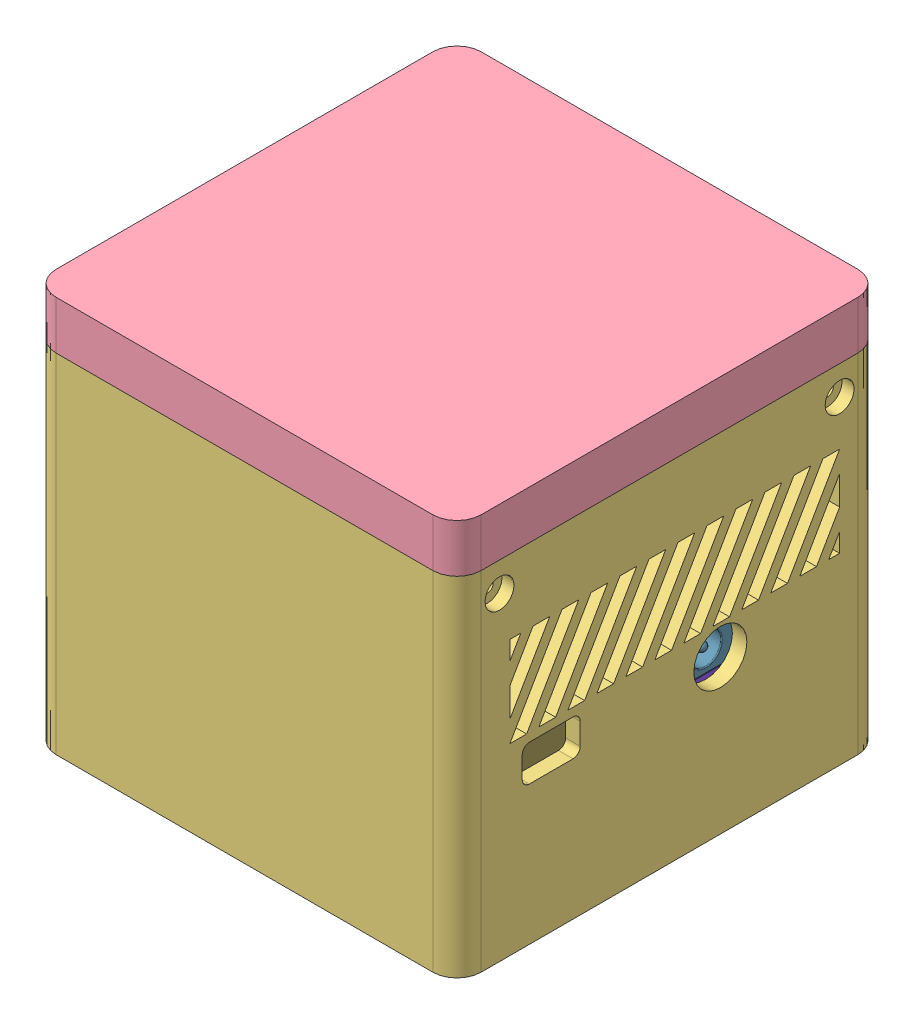
SolidWorks assembly 1219 ControlBox version, configuration 預設. Lengths in mm.
Overall size (88 82 106.01).
42 component instances, 34 part files, 73 mates.
Components (placement in the parent):
- 1219 third floor-1: 1219 third floor [預設] at (8.7787 40.759 112.8702) x (1 0 0) z (0 0 -1) size (81.6 37.75 81.6)
- 1219 second floor-1: 1219 second floor [預設] at (8.7787 -23.241 112.8702) x (1 0 0) z (0 0 -1) size (81.6 8 81.6)
- 1219 ground-1: 1219 ground [預設] at (0.3623 -33.241 92.6228) size (88 72 88)
- 1219 roof-1: 1219 roof [預設] at (-3.5854 48.759 93.9882) x (1 0 0) z (0 0 -1) size (88 10 88)
- STM32 fixed board-1: STM32 fixed board [預設] at (7.9161 -18.241 103.3439) x (-1 0 0) z (0 1 0) size (70.08 30 1.8)
- The small Fixed board on the converter-1: The small Fixed board on the converter [預設] at (21.8123 17.059 74.3493) x (0 0 -1) z (-1 0 0) size (46.7 1.6 58.25)
- M3_20mm_pillar-1: M3_20mm_pillar [預設] at (12.0438 39.859 57) x (-0.990685 0 -0.13617) z (-0.13617 0 0.990685) size (6 22.8 6)
- M3_20mm_pillar-2: M3_20mm_pillar [預設] at (28.2938 39.859 87.2) x (0.837169 0 0.546944) z (0.546944 0 -0.837169) size (6 22.8 6)
- 12VLEDconnector-1: 12VLEDconnector [預設] at (41.8438 -2.8554 76.5711) x (0 1 0) z (-1 0 0) size (12 37 6.2)
- O2-1: O2 [預設] at (-12.6825 28.759 117.8445) x (-1 0 0) z (0 1 0) size (37 27 19)
- JQC3F-1: JQC3F [預設] at (-14.4789 35.759 60.4222) x (1 0 0.000244) z (0 -1 0) size (33.51 25.73 16.5)
- LM2596 DC to DC Buck Converter 3 A-1: LM2596 DC to DC Buck Converter 3 A [預設] at (20.1688 38.759 72.1) x (0 0 -1) z (-1 0 0) size (43.2 15.15 21.25)
  - LM2596 DC to DC Buck Converter 3 A.STEP-1: LM2596 DC to DC Buck Converter 3 A.STEP [預設] at origin size (43.2 15.15 21.25)
    - lm2596board.STEP-1: lm2596board.STEP [預設] at origin size (43.2 1.71 21.25)
    - smd100uF.STEP-1: smd100uF.STEP [預設] at (-17.25 2.55 0) x (0 0 -1) z (1 0 0) size (11.2 9.76 8.2)
    - smd220uF.STEP-1: smd220uF.STEP [預設] at (17.25 2.55 0) x (0 0 -1) z (1 0 0) size (11.2 9.76 8.2)
    - TrimmerW203.STEP-1: TrimmerW203.STEP [預設] at (4.6271 6.95 -9.1276) size (9.5 15.15 4.81)
    - smdS537diode.STEP-1: smdS537diode.STEP [預設] at (-9.35 1.75 8.875) x (-1 0 0) z (0 0 -1) size (6.5 2.06 2.5)
    - smdceramiccapacitor.STEP-1: smdceramiccapacitor.STEP [預設] at (-15 1.7 5.7969) x (0 0 1) z (-1 0 0) size (2.52 0.61 1.3)
    - smdceramiccapacitor.STEP-2: smdceramiccapacitor.STEP [預設] at (-1.3196 1.7 -5.2916) x (0 0 1) z (-1 0 0) size (2.52 0.61 1.3)
    - smdResistor331.STEP-1: smdResistor331.STEP [預設] at (-1.2696 1.7 -8.4665) x (0 0 1) z (-1 0 0) size (2.53 0.63 1.31)
    - smdResistor102.STEP-1: smdResistor102.STEP [預設] at (10.7771 1.7 -8.4665) x (0 0 -1) z (1 0 0) size (2.53 0.63 1.31)
    - smdLED.STEP-1: smdLED.STEP [預設] at (13.0521 1.75 -8.4701) x (0 0 -1) z (1 0 0) size (3.23 0.86 1.26)
    - smbInductor470.STEP-1: smbInductor470.STEP [預設] at (3.1271 2.1 3.175) size (12.5 7.41 12.5)
    - LM2596S.STEP-1: LM2596S.STEP [預設] at (-8.0627 1.8 -4.5407) size (9.8 4.61 14.95)
- SCD30_CO2-1: SCD30_CO2 [預設] at (27.7597 38.759 111.9487) x (1 0 0) z (0 -1 0) size (35 23 13)
- Gravity Dissolved Oxygen Sensor v1.0.step-1: Gravity Dissolved Oxygen Sensor v1.0.step [預設] at (20.5726 -17.241 68.5206) x (-0.001647 0 0.999999) z (0 1 0) size (63.5 32 13.2)
- PH-4502C.STEP-1: PH-4502C.STEP [預設] at (-10.49 -8.3658 14.8331) x (0.023795 0 -0.999717) z (0.999717 0 0.023795) size (69.21 20.03 32.26)
  - Board_ph.STEP-1: Board_ph.STEP [預設] at (-41.1248 -11.8752 -79.7631) size (42 1.6 32)
  - BNC_90.STEP-1: BNC_90.STEP [預設] at (-42.729 11.0976 0.372) x (-0.000016 0 -1) z (0 -1 0) size (13 30 18)
  - Trimpot multivoltas_Valor predeterminado.STEP-1: Trimpot multivoltas_Valor predeterminado.STEP [預設] at (-58.9938 -5.1252 9.5069) x (-1 0 0) z (0 0 -1) size (9.8 15.4 5)
  - Trimpot multivoltas_Valor predeterminado.STEP-2: Trimpot multivoltas_Valor predeterminado.STEP [預設] at (-44.5735 -5.1252 13.9129) size (9.8 15.4 5)
  - pin_header_6.STEP-1: pin_header_6.STEP [預設] at (-71.799 -14.5822 4.6019) size (10.45 8.64 15.24)
  - S08.stp.STEP-1: S08.stp.STEP [預設] at (-63.5983 -10.4552 -1.493) x (1 0 0) z (0 1 0) size (4.9 6 1.55)
  - S08.stp.STEP-2: S08.stp.STEP [預設] at (-47.5601 -10.4552 -15.9552) x (-0.008727 0 0.999962) z (0 1 0) size (4.9 6 1.55)
  - S08.stp.STEP-3: S08.stp.STEP [預設] at (-45.4779 -10.4552 -0.8959) x (-0.999848 0 -0.017452) z (0 1 0) size (4.9 6 1.55)
  - ptc.STEP-1: ptc.STEP [預設] at (-58.5127 -8.5499 -13.3623) x (0 -1 0) z (0 0 -1) size (11.73 9.76 5.87)
- STM32 Nucleo-32-1: STM32 Nucleo-32 [預設] at (17.5119 -16.441 114.2714) x (1 0 0) z (0 1 0) size (50.29 18.54 16)
- JQC3F -2-1: JQC3F -2 [預設] at (-15.4815 35.759 86.544) x (1 0 0.000244) z (0 -1 0) size (34 26.5 16.5)
- DC socket-1: DC socket [Default] at (45.0438 -1.491 76.492) x (0 1 0) z (1 0 0) size (9.4 15 14.3)
- YELLOW JST XH 3 PIN CONNECTOR - P 2.54mm - ANGLED.stp-1: YELLOW JST XH 3 PIN CONNECTOR - P 2.54mm - ANGLED.stp [預設] at (19.2438 12.609 53.8153) x (0 -1 0) z (1 0 0) size (8.73 7.46 10.34)
- YELLOW JST XH 4 PIN CONNECTOR - P 2.54mm - ANGLED.stp-1: YELLOW JST XH 4 PIN CONNECTOR - P 2.54mm - ANGLED.stp [預設] at (-12.5062 12.609 53.8153) x (0 -1 0) z (1 0 0) size (8.73 7.46 12.88)
Mates (geometry in assembly coordinates):
- 重合/共線/共點6: coincident anti-aligned: plane of 1219 ground-1 through (0.3623 -25.241 92.6228) normal (0 1 0); plane of 1219 second floor-1 through (8.7787 -25.241 112.8702) normal (0 -1 0)
- 重合/共線/共點8: coincident anti-aligned: plane of 1219 second floor-1 through (8.7787 -23.241 112.8702) normal (0 1 0); plane of EC and PH support-1 through (-14.5186 -23.241 69.2115) normal (0 -1 0)
- 重合/共線/共點9: coincident anti-aligned: plane of EC and PH support-2 through (26.7761 -17.241 71.7105) normal (0 1 0); plane of Gravity Dissolved Oxygen Sensor v1.0.step-1 through (20.5726 -17.241 68.5206) normal (0 -1 0)
- 同軸心1: concentric aligned: cylinder of 1219 second floor-1 through (8.0438 -23.24 86) axis (0 -1 0) radius 1.2; cylinder of Gravity Dissolved Oxygen Sensor v1.0.step-1 through (8.0438 -15.741 86) axis (0 -1 0) radius 1.5
- 重合/共線/共點10: coincident anti-aligned: plane of EC and PH support-1 through (-14.5186 -20.241 69.2115) normal (0 1 0); plane of PH-4502C.STEP-1/Board_ph.STEP-1 through (1.9974 -20.241 47.1083) normal (0 -1 0)
- 同軸心3: concentric aligned: cylinder of 1219 second floor-1 through (-0.9062 -23.24 85.05) axis (0 -1 0) radius 1.2; cylinder of PH-4502C.STEP-1/Board_ph.STEP-1 through (-0.9062 -18.641 85.05) axis (0 -1 0) radius 1.5
- 重合/共線/共點16: coincident anti-aligned: plane of STM32 fixed board-1 through (7.9161 -16.441 103.3439) normal (0 1 0); plane of STM32 Nucleo-32-1 through (17.5119 -16.441 114.2714) normal (0 -1 0)
- 同軸心13: concentric aligned: cylinder of 1219 third floor-1 through (-24.9562 40.759 124) axis (0 -1 0) radius 1.2; cylinder of O2-1 through (-24.9562 30.759 124) axis (0 -1 0) radius 1.6
- 同軸心17: concentric aligned: cylinder of 1219 third floor-1 through (2.0438 40.759 50) axis (0 -1 0) radius 1.2; circle of JQC3F-1
- 同軸心18: concentric anti-aligned: cylinder of 1219 third floor-1 through (2.0438 40.759 70.5) axis (0 -1 0) radius 1.2; cylinder of JQC3F-1 through (2.0438 34.259 70.5) axis (0 1 0) radius 1.5
- 重合/共線/共點20: coincident anti-aligned: plane of 1219 third floor-1 through (8.7787 38.759 112.8702) normal (0 -1 0); plane of SCD30_CO2-1 through (27.7597 38.759 111.9487) normal (0 1 0)
- 同軸心21: concentric aligned: cylinder of 1219 third floor-1 through (11.0938 40.759 115.5) axis (0 -1 0) radius 1; cylinder of SCD30_CO2-1 through (11.0938 38.76 115.5) axis (0 -1 0) radius 0.875
- 同軸心22: concentric aligned: cylinder of 1219 third floor-1 through (43.0438 40.759 99.31) axis (0 -1 0) radius 1; cylinder of SCD30_CO2-1 through (43.0438 38.76 99.31) axis (0 -1 0) radius 0.875
- 同軸心23: concentric anti-aligned: circle of 1219 third floor-1; cylinder of LM2596 DC to DC Buck Converter 3 A-1/LM2596 DC to DC Buck Converter 3 A.STEP-1/lm2596board.STEP-1 through (12.0438 37.059 57) axis (0 1 0) radius 1.475
- 同軸心24: concentric aligned: cylinder of 1219 third floor-1 through (28.2938 40.759 87.2) axis (0 -1 0) radius 1.2; circle of LM2596 DC to DC Buck Converter 3 A-1/LM2596 DC to DC Buck Converter 3 A.STEP-1/lm2596board.STEP-1
- 重合/共線/共點27: coincident anti-aligned: plane of 1219 second floor-1 through (8.7787 -23.241 112.8702) normal (0 1 0); plane of EC and PH support-3 through (25.441 -23.241 60.8804) normal (0 -1 0)
- 重合/共線/共點28: coincident anti-aligned: plane of EC and PH support-2 through (26.7761 -20.241 71.7105) normal (0 -1 0); plane of EC and PH support-3 through (25.441 -20.241 60.8804) normal (0 1 0)
- 同軸心27: concentric aligned: cylinder of LM2596 DC to DC Buck Converter 3 A-1/LM2596 DC to DC Buck Converter 3 A.STEP-1/lm2596board.STEP-1 through (12.0438 37.059 57) axis (0 1 0) radius 1.475; cylinder of The small Fixed board on the converter-1 through (12.0438 15.459 57) axis (0 1 0) radius 1.5
- 同軸心28: concentric aligned: cylinder of LM2596 DC to DC Buck Converter 3 A-1/LM2596 DC to DC Buck Converter 3 A.STEP-1/lm2596board.STEP-1 through (28.2938 37.059 87.2) axis (0 1 0) radius 1.475; cylinder of The small Fixed board on the converter-1 through (28.2938 15.459 87.2) axis (0 1 0) radius 1.5
- 同軸心29: concentric aligned: cylinder of LM2596 DC to DC Buck Converter 3 A-1/LM2596 DC to DC Buck Converter 3 A.STEP-1/lm2596board.STEP-1 through (12.0438 37.059 57) axis (0 1 0) radius 1.475; cylinder of M3_20mm_pillar-1 through (12.0438 37.059 57) axis (0 1 0) radius 1.5
- 重合/共線/共點29: coincident anti-aligned: plane of LM2596 DC to DC Buck Converter 3 A-1/LM2596 DC to DC Buck Converter 3 A.STEP-1/lm2596board.STEP-1 through (20.1688 37.059 72.1) normal (0 -1 0); plane of M3_20mm_pillar-1 through (12.0438 37.059 57) normal (0 1 0)
- 同軸心30: concentric aligned: cylinder of LM2596 DC to DC Buck Converter 3 A-1/LM2596 DC to DC Buck Converter 3 A.STEP-1/lm2596board.STEP-1 through (28.2938 37.059 87.2) axis (0 1 0) radius 1.475; cylinder of M3_20mm_pillar-2 through (28.2938 37.059 87.2) axis (0 1 0) radius 1.5
- 重合/共線/共點30: coincident anti-aligned: plane of LM2596 DC to DC Buck Converter 3 A-1/LM2596 DC to DC Buck Converter 3 A.STEP-1/lm2596board.STEP-1 through (20.1688 37.059 72.1) normal (0 -1 0); plane of M3_20mm_pillar-2 through (28.2938 37.059 87.2) normal (0 1 0)
- 重合/共線/共點31: coincident anti-aligned: plane of The small Fixed board on the converter-1 through (21.8123 17.059 74.3493) normal (0 1 0); plane of M3_20mm_pillar-2 through (28.2938 17.059 87.2) normal (0 -1 0)
- 同軸心31: concentric anti-aligned: cylinder of The small Fixed board on the converter-1 through (28.2938 15.459 87.2) axis (0 1 0) radius 1.5; circle of M3_15mm_pillar-2
- 同軸心32: concentric anti-aligned: cylinder of The small Fixed board on the converter-1 through (12.0438 15.459 57) axis (0 1 0) radius 1.5; circle of M3_15mm_pillar-1
- 重合/共線/共點32: coincident anti-aligned: plane of The small Fixed board on the converter-1 through (21.8123 15.459 74.3493) normal (0 -1 0); plane of YELLOW JST XH 4 PIN CONNECTOR - P 2.54mm - ANGLED-1 through (14.0738 15.459 53.7353) normal (0 1 0)
- 重合/共線/共點35: coincident anti-aligned: plane of The small Fixed board on the converter-1 through (21.8123 15.459 74.3493) normal (0 -1 0); plane of YELLOW JST XH 4 PIN CONNECTOR - P 2.54mm - ANGLED-2 through (-18.8662 15.459 53.7353) normal (0 1 0)
- 重合/共線/共點38: coincident anti-aligned: plane of The small Fixed board on the converter-1 through (21.8123 15.459 74.3493) normal (0 -1 0); plane of YELLOW JST XH 4 PIN CONNECTOR - P 2.54mm - ANGLED-3 through (30.7938 15.459 86.7) normal (0 1 0)
- 重合/共線/共點39: coincident aligned: plane of The small Fixed board on the converter-1 through (30.7938 15.459 93.7) normal (0 0 1); plane of YELLOW JST XH 4 PIN CONNECTOR - P 2.54mm - ANGLED-3 through (24.3538 12.609 93.7) normal (0 0 1)
- 重合/共線/共點40: coincident aligned: plane of The small Fixed board on the converter-1 through (30.7938 15.459 93.7) normal (1 0 0); plane of YELLOW JST XH 4 PIN CONNECTOR - P 2.54mm - ANGLED-3 through (30.7938 9.759 86.7) normal (1 0 0)
- 重合/共線/共點44: coincident anti-aligned: plane of The small Fixed board on the converter-1 through (21.8123 15.459 74.3493) normal (0 -1 0); plane of YELLOW JST XH 4 PIN CONNECTOR - P 2.54mm - ANGLED-4 through (16.5438 15.459 93.7) normal (0 1 0)
- 重合/共線/共點45: coincident aligned: plane of The small Fixed board on the converter-1 through (9.5438 15.459 93.7) normal (-1 0 0); plane of YELLOW JST XH 4 PIN CONNECTOR - P 2.54mm - ANGLED-4 through (9.5438 12.609 87.26) normal (-1 0 0)
- 重合/共線/共點46: coincident aligned: plane of The small Fixed board on the converter-1 through (30.7938 15.459 93.7) normal (0 0 1); plane of YELLOW JST XH 4 PIN CONNECTOR - P 2.54mm - ANGLED-4 through (16.5438 9.759 93.7) normal (0 0 1)
- 同軸心34: concentric aligned: cylinder of 1219 third floor-1 through (41.9438 40.759 89.992) axis (0 -1 0) radius 1.2; cylinder of 12VLEDconnector-1 through (41.9438 3.01 89.992) axis (0 -1 0) radius 1.625
- 同軸心35: concentric aligned: cylinder of 1219 third floor-1 through (41.9438 40.759 62.992) axis (0 -1 0) radius 1.2; cylinder of 12VLEDconnector-1 through (41.9438 3.01 62.992) axis (0 -1 0) radius 1.625
- 同軸心41: concentric anti-aligned: cylinder of 1219 third floor-1 through (-26.9562 40.759 97) axis (0 -1 0) radius 1.2; cylinder of JQC3F -2-1 through (-26.9562 34.259 97) axis (0 1 0) radius 1.5
- 同軸心42: concentric anti-aligned: cylinder of 1219 third floor-1 through (-26.9562 40.759 76.5) axis (0 -1 0) radius 1.2; cylinder of JQC3F -2-1 through (-26.9562 34.259 76.5) axis (0 1 0) radius 1.5
- 重合/共線/共點52: coincident anti-aligned: plane of 1219 third floor-1 through (8.7787 38.759 112.8702) normal (0 -1 0); plane of LM2596 DC to DC Buck Converter 3 A-1/LM2596 DC to DC Buck Converter 3 A.STEP-1/lm2596board.STEP-1 through (20.1688 38.759 72.1) normal (0 1 0)
- 重合/共線/共點53: coincident anti-aligned: plane of 1219 third floor-1 through (8.7787 3.009 112.8702) normal (0 -1 0); plane of 12VLEDconnector-1 through (38.8438 3.009 67.992) normal (0 1 0)
- 重合/共線/共點61: coincident anti-aligned: plane of 1219 third floor-1 through (8.7787 3.009 112.8702) normal (0 -1 0); plane of DC socket-1 through (41.7438 3.009 81.992) normal (0 1 0)
- 重合/共線/共點62: coincident aligned: plane of 12VLEDconnector-1 through (45.0438 -2.8554 76.5711) normal (1 0 0); plane of DC socket-1 through (45.0438 -1.491 76.492) normal (1 0 0)
- 重合/共線/共點63: coincident anti-aligned: plane of 12VLEDconnector-1 through (38.8438 -1.491 81.992) normal (0 0 -1); plane of DC socket-1 through (41.7438 -5.991 81.992) normal (0 0 1)
- 重合/共線/共點74: coincident anti-aligned: plane of 1219 ground-1 through (0.3623 -25.241 92.6228) normal (0 1 0); plane of 1219 second floor-1 through (8.7787 -25.241 112.8702) normal (0 -1 0)
- 重合/共線/共點77: coincident aligned: plane of STM32 fixed board-1 through (42.3438 -16.441 126.4) normal (1 0 0); plane of STM32 Nucleo-32-1 through (42.3438 -0.441 102.4077) normal (1 0 0)
- 重合/共線/共點83: coincident aligned: plane of 1219 ground-1 through (-39.9562 -30.241 132) normal (0 0 1); plane of 1219 roof-1 through (-39.9562 45.759 132) normal (0 0 1)
- 重合/共線/共點84: coincident aligned: plane of 1219 ground-1 through (48.0438 -30.241 44) normal (1 0 0); plane of 1219 roof-1 through (48.0438 45.759 132) normal (1 0 0)
- 同軸心64: concentric aligned: circle of 1219 third floor-1; circle of 1219 roof-1
- 同軸心66: concentric aligned: cylinder of 1219 third floor-1 through (32.0438 40.76 124) axis (0 -1 0) radius 1.5; circle of 1219 roof-1
- 重合/共線/共點90: coincident anti-aligned: plane of 1219 third floor-1 through (8.7787 40.759 112.8702) normal (0 1 0); plane of 1219 roof-1 through (-3.5854 40.759 93.9882) normal (0 -1 0)
- 重合/共線/共點91: coincident anti-aligned: plane of 1219 ground-1 through (0.3623 38.759 92.6228) normal (0 1 0); plane of 1219 roof-1 through (-3.5854 38.759 93.9882) normal (0 -1 0)
- 同軸心67: concentric aligned: cylinder of 1219 third floor-1 through (4.8438 40.759 124) axis (0 -1 0) radius 1.2; cylinder of O2-1 through (4.8438 30.759 124) axis (0 -1 0) radius 1.6
- 同軸心68: concentric aligned: cylinder of 1219 third floor-1 through (4.8438 40.759 104) axis (0 -1 0) radius 1.2; cylinder of O2-1 through (4.8438 30.759 104) axis (0 -1 0) radius 1.6
- 重合/共線/共點92: coincident anti-aligned: plane of 1219 third floor-1 through (4.8438 30.759 124) normal (0 -1 0); plane of O2-1 through (-12.6825 30.759 117.8445) normal (0 1 0)
- 重合/共線/共點93: coincident anti-aligned: plane of 1219 third floor-1 through (-26.9562 35.759 97) normal (0 -1 0); plane of JQC3F -2-1 through (-15.4815 35.759 86.544) normal (0 1 0)
- 重合/共線/共點94: coincident anti-aligned: plane of 1219 third floor-1 through (-25.9562 35.759 70.5) normal (0 -1 0); plane of JQC3F-1 through (-14.4789 35.759 60.4222) normal (0 1 0)
- 同軸心69: concentric anti-aligned: circle of 1219 ground-1; circle of 1219 second floor-1
- 同軸心70: concentric anti-aligned: circle of 1219 ground-1; circle of 1219 second floor-1
- 重合/共線/共點95: coincident anti-aligned: plane of The small Fixed board on the converter-1 through (19.6338 17.459 53.5753) normal (0 0 1); plane of YELLOW JST XH 4 PIN CONNECTOR - P 2.54mm - ANGLED-1 through (16.3938 12.719 53.5753) normal (0 0 -1)
- 重合/共線/共點96: coincident: line of The small Fixed board on the converter-1 through (18.9338 17.059 53.5753) axis (1 0 0); plane of YELLOW JST XH 4 PIN CONNECTOR - P 2.54mm - ANGLED-1 through (16.3938 12.719 53.5753) normal (0 0 -1)
- 重合/共線/共點97: coincident: plane of The small Fixed board on the converter-1 through (16.3938 17.459 54.2753) normal (1 0 0); line of YELLOW JST XH 4 PIN CONNECTOR - P 2.54mm - ANGLED-1 through (16.3938 12.719 53.5753) axis (0 1 0)
- 重合/共線/共點98: coincident anti-aligned: plane of The small Fixed board on the converter-1 through (-18.4662 17.459 53.5753) normal (0 0 1); plane of YELLOW JST XH 4 PIN CONNECTOR - P 2.54mm - ANGLED-2 through (-8.3062 12.719 53.5753) normal (0 0 -1)
- 重合/共線/共點99: coincident: line of The small Fixed board on the converter-1 through (-8.3062 17.059 53.5753) axis (0 0 1); plane of YELLOW JST XH 4 PIN CONNECTOR - P 2.54mm - ANGLED-2 through (-8.3062 11.759 52.2353) normal (1 0 0)
- 重合/共線/共點105: coincident anti-aligned: plane of The small Fixed board on the converter-1 through (21.8123 15.459 74.3493) normal (0 -1 0); plane of JST-XH_3V_SMD.step-1/JST-XH_4-PIN.step-1 through (17.8738 15.459 54.1645) normal (0 1 0)
- 重合/共線/共點106: coincident anti-aligned: plane of The small Fixed board on the converter-1 through (18.9338 17.459 54.2753) normal (1 0 0); plane of JST-XH_3V_SMD.step-1/JST-XH_4-PIN.step-1 through (18.9338 14.9085 50.5078) normal (-1 0 0)
- 重合/共線/共點107: coincident: line of The small Fixed board on the converter-1 through (18.9338 17.059 53.5753) axis (1 0 0); plane of JST-XH_3V_SMD.step-1/JST-XH_4-PIN.step-1 through (19.5538 18.158 53.5945) normal (0 0.017452 -0.999848)
- 重合/共線/共點108: coincident anti-aligned: plane of The small Fixed board on the converter-1 through (21.8123 15.459 74.3493) normal (0 -1 0); plane of JST-XH_4V_SMD.step-1/JST-XH_4-PIN.step-1 through (1.0616 15.459 51.0661) normal (0 1 0)
- 重合/共線/共點112: coincident anti-aligned: plane of The small Fixed board on the converter-1 through (21.8123 15.459 74.3493) normal (0 -1 0); plane of YELLOW JST XH 3 PIN CONNECTOR - P 2.54mm - ANGLED.stp-1 through (14.0738 15.459 53.8153) normal (0 1 0)
- 重合/共線/共點114: coincident anti-aligned: plane of The small Fixed board on the converter-1 through (24.7138 17.459 54.2753) normal (0 0 -1); plane of YELLOW JST XH 3 PIN CONNECTOR - P 2.54mm - ANGLED.stp-1 through (21.4738 12.719 54.2753) normal (0 0 1)
- 重合/共線/共點116: coincident anti-aligned: plane of The small Fixed board on the converter-1 through (16.3938 17.459 54.2753) normal (1 0 0); plane of YELLOW JST XH 3 PIN CONNECTOR - P 2.54mm - ANGLED.stp-1 through (16.3938 12.379 52.3153) normal (-1 0 0)
- 重合/共線/共點117: coincident anti-aligned: plane of The small Fixed board on the converter-1 through (21.8123 15.459 74.3493) normal (0 -1 0); plane of YELLOW JST XH 4 PIN CONNECTOR - P 2.54mm - ANGLED.stp-1 through (-18.9462 15.459 53.8153) normal (0 1 0)
- 重合/共線/共點118: coincident anti-aligned: plane of The small Fixed board on the converter-1 through (-18.4662 17.459 54.2753) normal (0 0 -1); plane of YELLOW JST XH 4 PIN CONNECTOR - P 2.54mm - ANGLED.stp-1 through (-16.0062 12.719 54.2753) normal (0 0 1)
- 重合/共線/共點120: coincident anti-aligned: plane of The small Fixed board on the converter-1 through (-16.6262 17.459 54.2753) normal (1 0 0); plane of YELLOW JST XH 4 PIN CONNECTOR - P 2.54mm - ANGLED.stp-1 through (-16.6262 12.379 52.3153) normal (-1 0 0)
